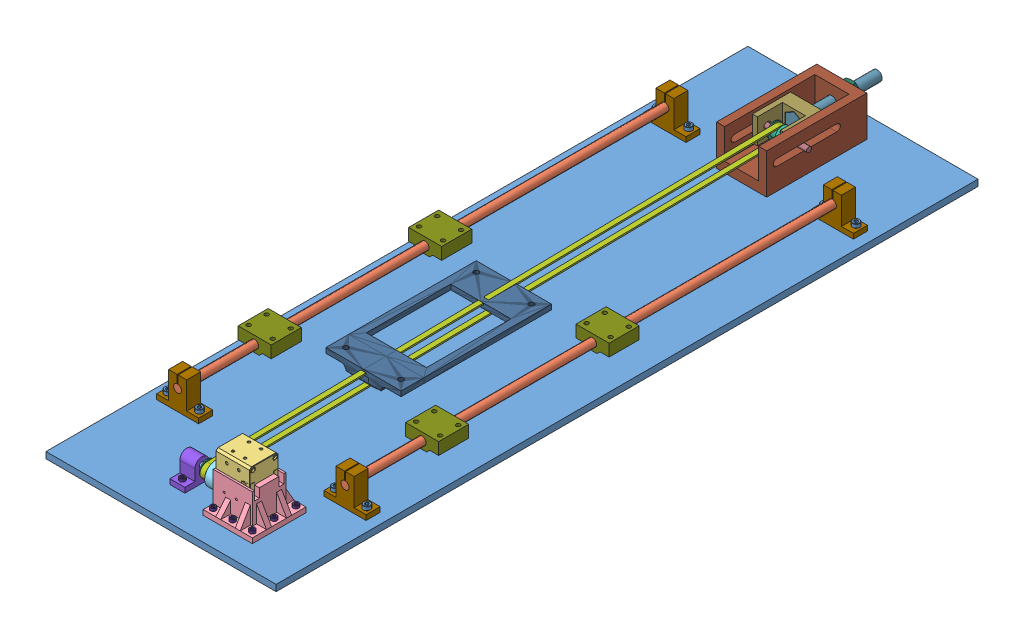
SolidWorks assembly linear_axis, configuration Défaut. Lengths in mm.
Overall size (229.5 66.71 714.21).
69 component instances, 25 part files, 88 mates.
Components (placement in the parent):
- plate-1: plate [Défaut] at origin size (229.5 6.35 700)
- rail-1: rail [Défaut] at (-83.5 26.35 250) x (-0.983228 -0.182381 0) z (0.182381 -0.983228 0) size (8 500 8)
- rail-2: rail [Défaut] at (83.5 26.35 250) x (0.983228 -0.182381 0) z (0.182381 0.983228 0) size (8 500 8)
- motor_case_pulley-1: motor_case_pulley [Défaut] at (16.75 22.6 300) x (0 0 1) z (-1 0 0) size (53.5 51.5 72)
  - XL430-W250-1: XL430-W250 [Défaut] at origin size (28.5 46.5 36.18)
  - motor_case-1: motor_case [Défaut] at (0 -16.25 -21.5) size (53.5 34.81 49)
  - coupler_pulley-2: coupler_pulley [Défaut] x (-1 0 0) z (0 1 0) size (22.5 12 20.75)
  - pulley-1: pulley [Défaut] at (0 0 21) x (1 0 0) z (0 1 0) size (15 16 15)
  - M2-4mm_TYPE 18-8 SS SOCKET HEAD CAP SCREW-1: M2-4mm_TYPE 18-8 SS SOCKET HEAD CAP SCREW [91292A832] at (-8 0 -2) x (-0.92231 0.38645 0) z (0 0 -1) size (3.8 3.8 6.09)
  - M2-4mm_TYPE 18-8 SS SOCKET HEAD CAP SCREW-2: M2-4mm_TYPE 18-8 SS SOCKET HEAD CAP SCREW [91292A832] at (0 8 -2) x (0.574993 -0.818158 0) z (0 0 -1) size (3.8 3.8 6.09)
  - M2-4mm_TYPE 18-8 SS SOCKET HEAD CAP SCREW-3: M2-4mm_TYPE 18-8 SS SOCKET HEAD CAP SCREW [91292A832] at (8 0 -2) x (-0.577346 0.816499 0) z (0 0 -1) size (3.8 3.8 6.09)
- pulley_axis_support-1: pulley_axis_support [Défaut] at (-9.25 22.6 300) x (0 0 1) z (0 -1 0) size (34 15 23)
- rail_support-5: rail_support [Défaut] at (-83.5 6.35 243) x (-1 0 0) z (0 0 -1) size (42 32 14)
- rail_support-6: rail_support [Défaut] at (83.5 6.35 243) x (-1 0 0) z (0 0 -1) size (42 32 14)
- rail_support-9: rail_support [Défaut] at (-83.5 6.35 -243) size (42 32 14)
- rail_support-10: rail_support [Défaut] at (83.5 6.35 -243) size (42 32 14)
- coupler_timing_belt_base-1: coupler_timing_belt_base [Défaut] at (37.5 33.85 148.1403) x (0 0 -1) z (-1 0 0) size (150 12 75)
- belt_tensioner-1: belt_tensioner [Défaut] at (70 26.35 -273.3415) x (0 0 1) z (-1 0 0) size (135.21 40 60)
  - tensioner_fixed_part-1: tensioner_fixed_part [Défaut] at (-5.6585 -20 70) size (100 40 50)
  - tensioner_moving_part-1: tensioner_moving_part [Défaut] at (17.1303 -7.5 53.5) size (38 25 33)
  - pulley-1: pulley [Défaut] at (7.1303 5 74.5) x (-0.489878 -0.871791 0) z (0.871791 -0.489878 0) size (15 16 15)
  - pulley_long_shaft-1: pulley_long_shaft [Défaut] at (7.1303 5 40) x (-0.998966 -0.045468 0) z (-0.045468 0.998966 0) size (5 60 5)
  - M10-75mm_TYPE 18-8 SS HEX HEAD CAP SCREW-1: M10-75mm_TYPE 18-8 SS HEX HEAD CAP SCREW [Défaut] at (-90.8697 5 70) x (0 -1 0) z (0 0 1) size (20 83 17.32)
  - M10-NUT_TYPE 18-8 SS THIN HEX NUT - DIN 439B (1)-1: M10-NUT_TYPE 18-8 SS THIN HEX NUT - DIN 439B (1) [Default] at (-55.6585 5 70) x (0 -0.532907 0.846174) z (0 -0.846174 -0.532907) size (17 10.59 19.63)
- linear_bearing-5: linear_bearing [Défaut] at (83.5 33.85 158.1403) x (-1 0 0) z (0 0 1) size (33 15 30)
- linear_bearing-6: linear_bearing [Défaut] at (83.5 33.85 -11.8597) x (-1 0 0) z (0 0 1) size (33 15 30)
- linear_bearing-7: linear_bearing [Défaut] at (-83.5 33.85 158.1403) x (1 0 0) z (0 0 -1) size (33 15 30)
- linear_bearing-8: linear_bearing [Défaut] at (-83.5 33.85 -11.8597) x (1 0 0) z (0 0 -1) size (33 15 30)
- M3-16mm_91292A115_TYPE 18-8 SS SOCKET HEAD CAP SCREW-1: M3-16mm_91292A115_TYPE 18-8 SS SOCKET HEAD CAP SCREW [91292A115] at (62.75 -4.65 321.75) x (0.995023 0 -0.099645) z (0 -1 0) size (5.5 5.5 19.25)
- M3-NUT_90710A030_TYPE 18-8 SS THIN HEX NUT - DIN 439B-1: M3-NUT_90710A030_TYPE 18-8 SS THIN HEX NUT - DIN 439B [90710A030] at (62.75 -0.9 321.75) x (0.992789 0 0.119878) z (-0.119878 0 0.992789) size (5.5 2.19 6.35)
- M3-NUT_90710A030_TYPE 18-8 SS THIN HEX NUT - DIN 439B-2: M3-NUT_90710A030_TYPE 18-8 SS THIN HEX NUT - DIN 439B [90710A030] at (43.25 -0.9 321.75) x (0.992789 0 0.119878) z (-0.119878 0 0.992789) size (5.5 2.19 6.35)
- M3-NUT_90710A030_TYPE 18-8 SS THIN HEX NUT - DIN 439B-3: M3-NUT_90710A030_TYPE 18-8 SS THIN HEX NUT - DIN 439B [90710A030] at (23.75 -0.9 321.75) x (0.992789 0 0.119878) z (-0.119878 0 0.992789) size (5.5 2.19 6.35)
- M3-16mm_91292A115_TYPE 18-8 SS SOCKET HEAD CAP SCREW-2: M3-16mm_91292A115_TYPE 18-8 SS SOCKET HEAD CAP SCREW [91292A115] at (43.25 -4.65 321.75) x (0.995023 0 -0.099645) z (0 -1 0) size (5.5 5.5 19.25)
- M3-16mm_91292A115_TYPE 18-8 SS SOCKET HEAD CAP SCREW-3: M3-16mm_91292A115_TYPE 18-8 SS SOCKET HEAD CAP SCREW [91292A115] at (23.75 -4.65 321.75) x (0.995023 0 -0.099645) z (0 -1 0) size (5.5 5.5 19.25)
- M3-NUT_90710A030_TYPE 18-8 SS THIN HEX NUT - DIN 439B-4: M3-NUT_90710A030_TYPE 18-8 SS THIN HEX NUT - DIN 439B [90710A030] at (62.75 -0.9 300) x (0.992789 0 0.119878) z (-0.119878 0 0.992789) size (5.5 2.19 6.35)
- M3-NUT_90710A030_TYPE 18-8 SS THIN HEX NUT - DIN 439B-5: M3-NUT_90710A030_TYPE 18-8 SS THIN HEX NUT - DIN 439B [90710A030] at (62.75 -0.9 278.25) x (0.992789 0 0.119878) z (-0.119878 0 0.992789) size (5.5 2.19 6.35)
- M3-16mm_91292A115_TYPE 18-8 SS SOCKET HEAD CAP SCREW-4: M3-16mm_91292A115_TYPE 18-8 SS SOCKET HEAD CAP SCREW [91292A115] at (62.75 -4.65 300) x (0.995023 0 -0.099645) z (0 -1 0) size (5.5 5.5 19.25)
- M3-16mm_91292A115_TYPE 18-8 SS SOCKET HEAD CAP SCREW-5: M3-16mm_91292A115_TYPE 18-8 SS SOCKET HEAD CAP SCREW [91292A115] at (62.75 -4.65 278.25) x (0.995023 0 -0.099645) z (0 -1 0) size (5.5 5.5 19.25)
- M3-NUT_90710A030_TYPE 18-8 SS THIN HEX NUT - DIN 439B-6: M3-NUT_90710A030_TYPE 18-8 SS THIN HEX NUT - DIN 439B [90710A030] at (43.25 -0.9 278.25) x (0.992789 0 0.119878) z (-0.119878 0 0.992789) size (5.5 2.19 6.35)
- M3-NUT_90710A030_TYPE 18-8 SS THIN HEX NUT - DIN 439B-7: M3-NUT_90710A030_TYPE 18-8 SS THIN HEX NUT - DIN 439B [90710A030] at (23.75 -0.9 278.25) x (0.992789 0 0.119878) z (-0.119878 0 0.992789) size (5.5 2.19 6.35)
- M3-16mm_91292A115_TYPE 18-8 SS SOCKET HEAD CAP SCREW-6: M3-16mm_91292A115_TYPE 18-8 SS SOCKET HEAD CAP SCREW [91292A115] at (43.25 -4.65 278.25) x (0.995023 0 -0.099645) z (0 -1 0) size (5.5 5.5 19.25)
- M3-16mm_91292A115_TYPE 18-8 SS SOCKET HEAD CAP SCREW-7: M3-16mm_91292A115_TYPE 18-8 SS SOCKET HEAD CAP SCREW [91292A115] at (23.75 -4.65 278.25) x (0.995023 0 -0.099645) z (0 -1 0) size (5.5 5.5 19.25)
- M3-16mm_91292A115_TYPE 18-8 SS SOCKET HEAD CAP SCREW-8: M3-16mm_91292A115_TYPE 18-8 SS SOCKET HEAD CAP SCREW [91292A115] at (-16.75 -4.4 312) x (0.715484 0 0.698629) z (0 -1 0) size (5.5 5.5 19.25)
- M3-NUT_90710A030_TYPE 18-8 SS THIN HEX NUT - DIN 439B-8: M3-NUT_90710A030_TYPE 18-8 SS THIN HEX NUT - DIN 439B [90710A030] at (-16.75 -0.9 312) size (5.5 2.19 6.35)
- M3-16mm_91292A115_TYPE 18-8 SS SOCKET HEAD CAP SCREW-9: M3-16mm_91292A115_TYPE 18-8 SS SOCKET HEAD CAP SCREW [91292A115] at (-16.75 -4.4 288) x (-0.715484 0 0.698629) z (0 -1 0) size (5.5 5.5 19.25)
- M3-NUT_90710A030_TYPE 18-8 SS THIN HEX NUT - DIN 439B-9: M3-NUT_90710A030_TYPE 18-8 SS THIN HEX NUT - DIN 439B [90710A030] at (-16.75 -0.9 288) size (5.5 2.19 6.35)
- M4-16mm_91292A118_TYPE 18-8 SS SOCKET HEAD CAP SCREW-1: M4-16mm_91292A118_TYPE 18-8 SS SOCKET HEAD CAP SCREW [91292A118] at (99.25 -4.65 244) x (0.684649 0 0.728873) z (0 -1 0) size (7 7 20.35)
- M4-16mm_91292A118_TYPE 18-8 SS SOCKET HEAD CAP SCREW-2: M4-16mm_91292A118_TYPE 18-8 SS SOCKET HEAD CAP SCREW [91292A118] at (67.75 -4.65 244) x (0.152759 0 0.988263) z (0 -1 0) size (7 7 20.35)
- M4-16mm_91292A118_TYPE 18-8 SS SOCKET HEAD CAP SCREW-3: M4-16mm_91292A118_TYPE 18-8 SS SOCKET HEAD CAP SCREW [91292A118] at (-99.25 -4.65 244) x (0.684649 0 -0.728873) z (0 -1 0) size (7 7 20.35)
- M4-16mm_91292A118_TYPE 18-8 SS SOCKET HEAD CAP SCREW-4: M4-16mm_91292A118_TYPE 18-8 SS SOCKET HEAD CAP SCREW [91292A118] at (-67.75 -4.65 244) x (0.152759 0 -0.988263) z (0 -1 0) size (7 7 20.35)
- M4-16mm_91292A118_TYPE 18-8 SS SOCKET HEAD CAP SCREW-5: M4-16mm_91292A118_TYPE 18-8 SS SOCKET HEAD CAP SCREW [91292A118] at (99.25 -4.65 -244) x (0.684649 0 -0.728873) z (0 -1 0) size (7 7 20.35)
- M4-16mm_91292A118_TYPE 18-8 SS SOCKET HEAD CAP SCREW-6: M4-16mm_91292A118_TYPE 18-8 SS SOCKET HEAD CAP SCREW [91292A118] at (67.75 -4.65 -244) x (-0.152759 0 0.988263) z (0 -1 0) size (7 7 20.35)
- M4-16mm_91292A118_TYPE 18-8 SS SOCKET HEAD CAP SCREW-7: M4-16mm_91292A118_TYPE 18-8 SS SOCKET HEAD CAP SCREW [91292A118] at (-99.25 -4.65 -244) x (-0.684649 0 -0.728873) z (0 -1 0) size (7 7 20.35)
- M4-16mm_91292A118_TYPE 18-8 SS SOCKET HEAD CAP SCREW-8: M4-16mm_91292A118_TYPE 18-8 SS SOCKET HEAD CAP SCREW [91292A118] at (-67.75 -4.65 -244) x (-0.152759 0 -0.988263) z (0 -1 0) size (7 7 20.35)
- M5-20mm_TYPE 18-8 SS SOCKET HEAD CAP SCREW-1: M5-20mm_TYPE 18-8 SS SOCKET HEAD CAP SCREW [91292A118] at (0 -8.65 -304) x (0.974897 0 -0.222657) z (0 -1 0) size (9 9 24.44)
- M5-20mm_TYPE 18-8 SS SOCKET HEAD CAP SCREW-2: M5-20mm_TYPE 18-8 SS SOCKET HEAD CAP SCREW [91292A118] at (0 -8.65 -279) x (0.302619 0 0.953112) z (0 -1 0) size (9 9 24.44)
- M4-NUT_90710A035_TYPE 18-8 SS THIN HEX NUT - DIN 439B-9: M4-NUT_90710A035_TYPE 18-8 SS THIN HEX NUT - DIN 439B [90710A035] at (99.25 -1.1 244) x (0.723417 0 0.690412) z (-0.690412 0 0.723417) size (7 2.75 8.08)
- M4-NUT_90710A035_TYPE 18-8 SS THIN HEX NUT - DIN 439B-10: M4-NUT_90710A035_TYPE 18-8 SS THIN HEX NUT - DIN 439B [90710A035] at (67.75 -1.1 244) x (0.272287 0 0.962216) z (-0.962216 0 0.272287) size (7 2.75 8.08)
- M4-NUT_90710A035_TYPE 18-8 SS THIN HEX NUT - DIN 439B-11: M4-NUT_90710A035_TYPE 18-8 SS THIN HEX NUT - DIN 439B [90710A035] at (-99.25 -1.1004 244) x (-0.723417 0 0.690412) z (0.690412 0 0.723417) size (7 2.75 8.08)
- M4-NUT_90710A035_TYPE 18-8 SS THIN HEX NUT - DIN 439B-12: M4-NUT_90710A035_TYPE 18-8 SS THIN HEX NUT - DIN 439B [90710A035] at (-67.75 -1.1004 244) x (-0.272287 0 0.962216) z (0.962216 0 0.272287) size (7 2.75 8.08)
- M4-NUT_90710A035_TYPE 18-8 SS THIN HEX NUT - DIN 439B-13: M4-NUT_90710A035_TYPE 18-8 SS THIN HEX NUT - DIN 439B [90710A035] at (99.25 -1.1004 -244) x (0.723417 0 -0.690412) z (-0.690412 0 -0.723417) size (7 2.75 8.08)
- M4-NUT_90710A035_TYPE 18-8 SS THIN HEX NUT - DIN 439B-14: M4-NUT_90710A035_TYPE 18-8 SS THIN HEX NUT - DIN 439B [90710A035] at (67.75 -1.1004 -244) x (0.272287 0 -0.962216) z (-0.962216 0 -0.272287) size (7 2.75 8.08)
- M4-NUT_90710A035_TYPE 18-8 SS THIN HEX NUT - DIN 439B-15: M4-NUT_90710A035_TYPE 18-8 SS THIN HEX NUT - DIN 439B [90710A035] at (-67.75 -1.1 -244) x (-0.272287 0 -0.962216) z (0.962216 0 -0.272287) size (7 2.75 8.08)
- M4-NUT_90710A035_TYPE 18-8 SS THIN HEX NUT - DIN 439B-16: M4-NUT_90710A035_TYPE 18-8 SS THIN HEX NUT - DIN 439B [90710A035] at (-99.25 -1.1 -244) x (-0.723417 0 -0.690412) z (0.690412 0 -0.723417) size (7 2.75 8.08)
- M5-NUT_TYPE 18-8 SS THIN HEX NUT - DIN 439B-9: M5-NUT_TYPE 18-8 SS THIN HEX NUT - DIN 439B [90710A035] at (0 -1.5 -304) x (0.987172 0 -0.159659) z (0.159659 0 0.987172) size (8 3.55 9.24)
- M5-NUT_TYPE 18-8 SS THIN HEX NUT - DIN 439B-10: M5-NUT_TYPE 18-8 SS THIN HEX NUT - DIN 439B [90710A035] at (0 -1.5 -279) size (8 3.55 9.24)
- pulley_shaft-1: pulley_shaft [Défaut] at (-23.4279 22.6 300) x (0 -0.50423 0.863569) z (0 0.863569 0.50423) size (5 40 5)
- M4-8mm_91292A108_TYPE 18-8 SS SOCKET HEAD CAP SCREW-1: M4-8mm_91292A108_TYPE 18-8 SS SOCKET HEAD CAP SCREW [91292A108] at (7.75 20.1 300) x (0.999637 0 -0.026942) z (0 1 0) size (7 7 12.31)
- timing_belt-1: timing_belt [Défaut] at (0 26.9744 17.7551) x (0 -0.015407 0.999881) z (1 0 0) size (582 14 5)
Mates (geometry in assembly coordinates):
- Parallèle2: parallel aligned: plane of plaque-1 through (114.75 6.35 -350) normal (1 0 0); plane of robot_base_plate-1 through (100 35.85 -91.2538) normal (1 0 0)
- Parallèle3: parallel anti-aligned: plane of plaque-1 through (0 6.35 0) normal (0 1 0); plane of robot_base_plate-1 through (0 33.85 8.7462) normal (0 -1 0)
- Largeur1: width anti-aligned: plane of robot_base_plate-1 through (100 35.85 -91.2538) normal (1 0 0); plane of plaque-1 through (-100 35.85 -91.2538) normal (-1 0 0); plane of robot_base_plate-1 through (-114.75 6.35 -350) normal (-1 0 0); plane of plaque-1 through (114.75 6.35 -350) normal (1 0 0)
- Coïncidente4: coincident anti-aligned: plane of robot_base_plate-1 through (0 33.85 8.7462) normal (0 -1 0); plane of linear_bearing-1 through (131.2296 66.0945 93.7462) normal (0 1 0)
- Coïncidente5: coincident: point of robot_base_plate-1; unknown of linear_bearing-1
- Coïncidente6: coincident aligned: plane of robot_base_plate-1 through (-100 35.85 108.7462) normal (0 0 1); plane of linear_bearing-1 through (114.7296 51.0945 108.7462) normal (0 0 1)
- Parallèle4: parallel aligned: plane of plaque-1 through (114.75 6.35 350) normal (0 0 1); plane of rail_cylindre-1 through (-83.5 26.35 250) normal (0 0 1)
- Coaxiale1: concentric aligned: circle of bearing_lineaire-2; circle of rail_cylindre-1
- Largeur2: width anti-aligned: plane of rail-1 through (-83.5 26.35 250) normal (0 0 1); plane of plaque-1 through (-83.5 26.35 -250) normal (0 0 -1); plane of rail-1 through (114.75 6.35 -350) normal (0 0 -1); plane of plaque-1 through (114.75 6.35 350) normal (0 0 1)
- Parallèle5: parallel: plane of plaque-1 through (-114.75 6.35 -350) normal (-1 0 0); line of moteuretsupport-1/support moteur-1 through (18.75 6.35 273.25) axis (0 0 1)
- Coïncidente15: coincident anti-aligned: plane of plaque-1 through (0 6.35 0) normal (0 1 0); plane of moteuretsupport-1/support moteur-1 through (38.25 6.35 300) normal (0 -1 0)
- Distance1: distance = 47 mm aligned: plane of plaque-1 through (114.75 6.35 -350) normal (1 0 0); plane of moteuretsupport-1/support moteur-1 through (67.75 11.35 273.25) normal (1 0 0)
- Distance2: distance = 50 mm: unknown of moteuretsupport-1/support moteur-1; line of plaque-1 through (-114.75 6.35 350) axis (1 0 0)
- Parallèle6: parallel anti-aligned: plane of plaque-1 through (0 6.35 0) normal (0 1 0); plane of support_axe_poulie-1 through (-24.25 6.6 283) normal (0 -1 0)
- Coaxiale2: concentric anti-aligned: circle of moteuretsupport-1/poulie-1; circle of support_axe_poulie-1
- Distance3: distance = 5 mm anti-aligned: plane of support_axe_poulie-1 through (-9.25 22.6 300) normal (1 0 0); plane of moteuretsupport-1/poulie-1 through (-4.25 22.6 300) normal (-1 0 0)
- Coïncidente19: coincident aligned: circle of rail_cylindre-1; circle of support_rail-5
- Coïncidente21: coincident anti-aligned: circle of plaque-1; circle of support_rail-5
- Coïncidente23: coincident aligned: circle of rail_cylindre-2; circle of support_rail-6
- Coïncidente24: coincident anti-aligned: circle of plaque-1; circle of support_rail-6
- Coïncidente25: coincident anti-aligned: circle of plaque-1; circle of support_rail-10
- Coïncidente26: coincident anti-aligned: circle of plaque-1; circle of support_rail-9
- Coïncidente28: coincident anti-aligned: circle of rail_cylindre-2; circle of support_rail-10
- Coïncidente30: coincident anti-aligned: circle of rail_cylindre-1; circle of support_rail-9
- Parallèle7: parallel anti-aligned: plane of robot_base_plate-1 through (-100 35.85 -91.2538) normal (0 0 -1); plane of coupler_timing_belt_base-1 through (37.5 33.85 148.1403) normal (0 0 1)
- Coïncidente32: coincident anti-aligned: plane of robot_base_plate-1 through (0 33.85 8.7462) normal (0 -1 0); plane of coupler_timing_belt_base-1 through (37.5 33.85 148.1403) normal (0 1 0)
- Largeur3: width anti-aligned: plane of coupler_timing_belt_base-1 through (37.5 33.85 -1.8597) normal (0 0 -1); plane of robot_base_plate-1 through (37.5 33.85 148.1403) normal (0 0 1); plane of coupler_timing_belt_base-1 through (-100 35.85 108.7462) normal (0 0 1); plane of robot_base_plate-1 through (-100 35.85 -91.2538) normal (0 0 -1)
- Largeur4: width anti-aligned: plane of coupler_timing_belt_base-1 through (37.5 33.85 148.1403) normal (1 0 0); plane of robot_base_plate-1 through (-37.5 33.85 148.1403) normal (-1 0 0); plane of coupler_timing_belt_base-1 through (-100 35.85 -91.2538) normal (-1 0 0); plane of robot_base_plate-1 through (100 35.85 -91.2538) normal (1 0 0)
- Parallèle9: parallel aligned: plane of plate-1 through (114.75 6.35 -350) normal (1 0 0); plane of belt_tensioner-1/tensioner_fixed_part-1 through (25 16.35 -329) normal (1 0 0)
- Coïncidente35: coincident anti-aligned: plane of plate-1 through (0 6.35 0) normal (0 1 0); plane of belt_tensioner-1/tensioner_fixed_part-1 through (0 6.35 -279) normal (0 -1 0)
- Coaxiale3: concentric aligned: cylinder of plate-1 through (0 0 -304) axis (0 1 0) radius 2.75; cylinder of belt_tensioner-1/tensioner_fixed_part-1 through (0 16.35 -304) axis (0 1 0) radius 2.75
- Coïncidente36: coincident anti-aligned: line of linear_bearing-1 through (147.7296 66.0945 78.7462) axis (0 0 1); line of Base_Robot-1 through (147.7296 66.0945 104.9261) axis (0 0 -1)
- Coaxiale4: concentric aligned: cylinder of rail-2 through (83.5 26.35 -250) axis (0 0 1) radius 4; circle of linear_bearing-5
- Parallèle10: parallel aligned: plane of plate-1 through (0 6.35 0) normal (0 1 0); plane of linear_bearing-5 through (83.5 33.85 158.1403) normal (0 1 0)
- Parallèle11: parallel aligned: plane of plate-1 through (0 6.35 0) normal (0 1 0); plane of linear_bearing-6 through (83.5 33.85 -11.8597) normal (0 1 0)
- Coaxiale5: concentric aligned: cylinder of rail-2 through (83.5 26.35 -250) axis (0 0 1) radius 4; cylinder of linear_bearing-6 through (83.5 26.35 -26.8597) axis (0 0 1) radius 4
- Coïncidente41: coincident anti-aligned: line of linear_bearing-5 through (100 33.85 143.1403) axis (0 0 1); line of robot_base_plate-2 through (100 33.85 70.7474) axis (0 0 -1)
- Coïncidente42: coincident anti-aligned: plane of linear_bearing-8 through (-83.5 33.85 -11.8597) normal (0 1 0); plane of robot_base_plate-2 through (0 33.85 -29.2526) normal (0 -1 0)
- Coïncidente43: coincident anti-aligned: line of linear_bearing-8 through (-100 33.85 -26.8597) axis (1 0 0); line of robot_base_plate-2 through (100 33.85 -129.2526) axis (-1 0 0)
- Coïncidente44: coincident anti-aligned: line of linear_bearing-7 through (-67 33.85 173.1403) axis (-1 0 0); line of robot_base_plate-2 through (-100 33.85 70.7474) axis (1 0 0)
- Coïncidente45: coincident anti-aligned: plane of coupler_timing_belt_base-1 through (37.5 33.85 148.1403) normal (0 1 0); plane of Base_Robot-2 through (0 33.85 -29.2526) normal (0 -1 0)
- Largeur5: width anti-aligned: plane of coupler_timing_belt_base-1 through (-37.5 33.85 148.1403) normal (-1 0 0); plane of coupler_timing_belt_base-1 through (37.5 33.85 148.1403) normal (1 0 0); plane of Base_Robot-2 through (100 35.85 70.7474) normal (1 0 0); plane of Base_Robot-2 through (-100 35.85 70.7474) normal (-1 0 0)
- Largeur6: width anti-aligned: plane of coupler_timing_belt_base-1 through (37.5 33.85 -1.8597) normal (0 0 -1); plane of coupler_timing_belt_base-1 through (37.5 33.85 148.1403) normal (0 0 1); plane of Base_Robot-2 through (100 35.85 70.7474) normal (0 0 1); plane of Base_Robot-2 through (100 35.85 -129.2526) normal (0 0 -1)
- Coïncidente47: coincident aligned: plane of coupler_timing_belt_base-1 through (37.5 33.85 148.1403) normal (0 1 0); plane of linear_bearing-7 through (-83.5 33.85 158.1403) normal (0 1 0)
- Largeur7: width anti-aligned: plane of coupler_timing_belt_base-1 through (37.5 33.85 148.1403) normal (1 0 0); plane of plate-1 through (-37.5 33.85 148.1403) normal (-1 0 0); plane of coupler_timing_belt_base-1 through (-114.75 6.35 -350) normal (-1 0 0); plane of plate-1 through (114.75 6.35 -350) normal (1 0 0)
- Distance4: distance = 200 mm: line of linear_bearing-7 through (-67 33.85 173.1403) axis (-1 0 0); line of linear_bearing-8 through (-100 33.85 -26.8597) axis (1 0 0)
- Largeur8: width anti-aligned: plane of coupler_timing_belt_base-1 through (37.5 33.85 148.1403) normal (0 0 1); plane of linear_bearing-6 through (37.5 33.85 -1.8597) normal (0 0 -1); plane of coupler_timing_belt_base-1 through (67 18.85 -26.8597) normal (0 0 -1); plane of linear_bearing-5 through (67 18.85 173.1403) normal (0 0 1)
- Coaxiale6: concentric anti-aligned: cylinder of motor_case_pulley-1/motor_case-1 through (62.75 6.35 321.75) axis (0 1 0) radius 2; cylinder of M3-12mm_91292A114_TYPE 18-8 SS SOCKET HEAD CAP SCREW-1 through (62.75 19.8774 321.75) axis (0 -1 0) radius 2.75
- Coaxiale7: concentric anti-aligned: cylinder of motor_case_pulley-1/motor_case-1 through (62.75 6.35 321.75) axis (0 1 0) radius 2; cylinder of M3-16mm_91292A115_TYPE 18-8 SS SOCKET HEAD CAP SCREW-1 through (62.75 14.35 321.75) axis (0 -1 0) radius 2.75
- Coïncidente50: coincident anti-aligned: plane of motor_case_pulley-1/motor_case-1 through (38.25 11.35 300) normal (0 1 0); plane of M3-16mm_91292A115_TYPE 18-8 SS SOCKET HEAD CAP SCREW-1 through (62.75 11.35 321.75) normal (0 -1 0)
- Coaxiale8: concentric anti-aligned: circle of plate-1; circle of M3-NUT_90710A030_TYPE 18-8 SS THIN HEX NUT - DIN 439B-1
- Coïncidente51: coincident anti-aligned: plane of plate-1 through (0 0 0) normal (0 -1 0); plane of M3-NUT_90710A030_TYPE 18-8 SS THIN HEX NUT - DIN 439B-1 through (60.2102 0 319.8441) normal (0 1 0)
- Coaxiale9: concentric anti-aligned: cylinder of pulley_axis_support-1 through (-16.75 -3.4 312) axis (0 1 0) radius 2; cylinder of M3-16mm_91292A115_TYPE 18-8 SS SOCKET HEAD CAP SCREW-8 through (-16.75 14.6 312) axis (0 -1 0) radius 2.75
- Coïncidente52: coincident anti-aligned: plane of pulley_axis_support-1 through (-24.25 11.6 307) normal (0 1 0); plane of M3-16mm_91292A115_TYPE 18-8 SS SOCKET HEAD CAP SCREW-8 through (-16.75 11.6 312) normal (0 -1 0)
- Coïncidente53: coincident anti-aligned: cylinder of M3-16mm_91292A115_TYPE 18-8 SS SOCKET HEAD CAP SCREW-8 through (-16.75 14.6 312) axis (0 -1 0) radius 2.75; circle of M3-NUT_90710A030_TYPE 18-8 SS THIN HEX NUT - DIN 439B-8
- Coïncidente54: coincident anti-aligned: plane of plate-1 through (0 0 0) normal (0 -1 0); plane of M3-NUT_90710A030_TYPE 18-8 SS THIN HEX NUT - DIN 439B-8 through (-19.5 0 310.4123) normal (0 1 0)
- Coaxiale10: concentric anti-aligned: cylinder of rail_support-6 through (99.25 6.35 244) axis (0 1 0) radius 2.5; cylinder of M4-16mm_91292A118_TYPE 18-8 SS SOCKET HEAD CAP SCREW-1 through (99.25 15.35 244) axis (0 -1 0) radius 3.5
- Coïncidente55: coincident anti-aligned: plane of rail_support-6 through (104.5 11.35 250) normal (0 1 0); plane of M4-16mm_91292A118_TYPE 18-8 SS SOCKET HEAD CAP SCREW-1 through (99.25 11.35 244) normal (0 -1 0)
- Coaxiale11: concentric anti-aligned: cylinder of rail_support-6 through (67.75 6.35 244) axis (0 1 0) radius 2.5; cylinder of M4-16mm_91292A118_TYPE 18-8 SS SOCKET HEAD CAP SCREW-2 through (67.75 15.35 244) axis (0 -1 0) radius 3.5
- Coïncidente56: coincident anti-aligned: plane of rail_support-6 through (62.5 11.35 250) normal (0 1 0); plane of M4-16mm_91292A118_TYPE 18-8 SS SOCKET HEAD CAP SCREW-2 through (67.75 11.35 244) normal (0 -1 0)
- Coaxiale12: concentric anti-aligned: cylinder of M4-16mm_91292A118_TYPE 18-8 SS SOCKET HEAD CAP SCREW-1 through (99.25 15.35 244) axis (0 -1 0) radius 3.5; circle of M4-NUT_90710A035_TYPE 18-8 SS THIN HEX NUT - DIN 439B-2
- Coïncidente58: coincident: cylinder of M4-16mm_91292A118_TYPE 18-8 SS SOCKET HEAD CAP SCREW-2 through (67.75 15.35 244) axis (0 -1 0) radius 3.5; circle of M4-NUT_90710A035_TYPE 18-8 SS THIN HEX NUT - DIN 439B-1
- Coïncidente59: coincident anti-aligned: plane of plate-1 through (0 0 0) normal (0 -1 0); plane of M5-NUT_TYPE 18-8 SS THIN HEX NUT - DIN 439B-2 through (95.9545 0 240.7638) normal (0 1 0)
- Coïncidente60: coincident: plane of plate-1 through (0 0 0) normal (0 -1 0); plane of M4-NUT_90710A035_TYPE 18-8 SS THIN HEX NUT - DIN 439B-1 through (63.75 0.4 241.6905) normal (0 1 0)
- Coaxiale14: concentric anti-aligned: cylinder of belt_tensioner-1/tensioner_fixed_part-1 through (0 16.35 -304) axis (0 1 0) radius 5; cylinder of M5-20mm_TYPE 18-8 SS SOCKET HEAD CAP SCREW-1 through (0 15.35 -304) axis (0 -1 0) radius 4.5
- Coïncidente62: coincident anti-aligned: plane of belt_tensioner-1/tensioner_fixed_part-1 through (0 11.35 -301.25) normal (0 1 0); plane of M5-20mm_TYPE 18-8 SS SOCKET HEAD CAP SCREW-1 through (0 11.35 -304) normal (0 -1 0)
- Coaxiale15: concentric anti-aligned: cylinder of belt_tensioner-1/tensioner_fixed_part-1 through (0 16.35 -279) axis (0 1 0) radius 5; cylinder of M5-20mm_TYPE 18-8 SS SOCKET HEAD CAP SCREW-2 through (0 15.35 -279) axis (0 -1 0) radius 4.5
- Coïncidente63: coincident anti-aligned: plane of belt_tensioner-1/tensioner_fixed_part-1 through (0 11.35 -276.25) normal (0 1 0); plane of M5-20mm_TYPE 18-8 SS SOCKET HEAD CAP SCREW-2 through (0 11.35 -279) normal (0 -1 0)
- Coïncidente64: coincident anti-aligned: cylinder of M4-16mm_91292A118_TYPE 18-8 SS SOCKET HEAD CAP SCREW-1 through (99.25 15.35 244) axis (0 -1 0) radius 3.5; circle of M4-NUT_90710A035_TYPE 18-8 SS THIN HEX NUT - DIN 439B-9
- Coïncidente65: coincident anti-aligned: plane of plate-1 through (0 0 0) normal (0 -1 0); plane of M4-NUT_90710A035_TYPE 18-8 SS THIN HEX NUT - DIN 439B-9 through (98.1132 0 240.1217) normal (0 1 0)
- Coïncidente66: coincident anti-aligned: cylinder of M4-16mm_91292A118_TYPE 18-8 SS SOCKET HEAD CAP SCREW-2 through (67.75 15.35 244) axis (0 -1 0) radius 3.5; circle of M4-NUT_90710A035_TYPE 18-8 SS THIN HEX NUT - DIN 439B-10
- Coïncidente67: coincident anti-aligned: plane of plate-1 through (0 0 0) normal (0 -1 0); plane of M4-NUT_90710A035_TYPE 18-8 SS THIN HEX NUT - DIN 439B-10 through (68.7414 0 240.082) normal (0 1 0)
- Coaxiale16: concentric aligned: circle of plate-1; circle of M5-NUT_TYPE 18-8 SS THIN HEX NUT - DIN 439B-9
- Coïncidente68: coincident anti-aligned: plane of plate-1 through (0 0 0) normal (0 -1 0); plane of M5-NUT_TYPE 18-8 SS THIN HEX NUT - DIN 439B-9 through (-4.3174 0 -305.6411) normal (0 1 0)
- Coïncidente69: coincident anti-aligned: plane of plate-1 through (0 0 0) normal (0 -1 0); plane of M5-NUT_TYPE 18-8 SS THIN HEX NUT - DIN 439B-10 through (-4 0 -281.3094) normal (0 1 0)
- Coaxiale17: concentric anti-aligned: circle of plate-1; circle of M5-NUT_TYPE 18-8 SS THIN HEX NUT - DIN 439B-10
- Coaxiale18: concentric anti-aligned: cylinder of pulley_axis_support-1 through (-24.25 22.6 300) axis (1 0 0) radius 2.5; cylinder of pulley_shaft-1 through (16.5721 22.6 300) axis (-1 0 0) radius 2.5
- Coïncidente70: coincident anti-aligned: plane of motor_case_pulley-1/XL430-W250-1 through (16.5721 27.1585 295) normal (-1 0 0); plane of pulley_shaft-1 through (16.5721 22.6 300) normal (1 0 0)
- Coaxiale19: concentric anti-aligned: cylinder of motor_case_pulley-1/coupler_pulley-2 through (7.75 23.1 300) axis (0 -1 0) radius 2; cylinder of M4-8mm_91292A108_TYPE 18-8 SS SOCKET HEAD CAP SCREW-1 through (7.75 8.1 300) axis (0 1 0) radius 3.5
- Tangent1: tangent anti-aligned: cylinder of pulley_shaft-1 through (16.5721 22.6 300) axis (-1 0 0) radius 2.5; plane of M4-8mm_91292A108_TYPE 18-8 SS SOCKET HEAD CAP SCREW-1 through (7.75 20.1 300) normal (0 1 0)
- Coaxiale20: concentric aligned: cylinder of belt_tensioner-1/tensioner_fixed_part-1 through (0 31.35 -229) axis (0 0 -1) radius 5.25; cylinder of M10-75mm_TYPE 18-8 SS HEX HEAD CAP SCREW-1 through (0 31.35 -290.6137) axis (0 0 -1) radius 5
- Coïncidente72: coincident anti-aligned: plane of belt_tensioner-1/tensioner_moving_part-1 through (16.5 18.85 -289.2112) normal (0 0 1); plane of M10-75mm_TYPE 18-8 SS HEX HEAD CAP SCREW-1 through (0 31.35 -290.6137) normal (0 0 -1)
- Parallèle12: parallel anti-aligned: plane of belt_tensioner-1/tensioner_moving_part-1 through (9.0933 36.6 -289.2112) normal (-0.5 -0.866025 0); plane of M10-75mm_TYPE 18-8 SS HEX HEAD CAP SCREW-1 through (0 41.35 -282.6137) normal (0.5 0.866025 0)
- Coaxiale21: concentric: cylinder of M10-75mm_TYPE 18-8 SS HEX HEAD CAP SCREW-1 through (0 31.35 -290.6137) axis (0 0 -1) radius 5; circle of M10-NUT_TYPE 18-8 SS THIN HEX NUT - DIN 439B (1)-1
- Coïncidente74: coincident anti-aligned: plane of belt_tensioner-1/tensioner_fixed_part-1 through (-25 16.35 -329) normal (0 0 -1); plane of M10-NUT_TYPE 18-8 SS THIN HEX NUT - DIN 439B (1)-1 through (0 31.35 -329) normal (0 0 1)
- Coaxiale22: concentric anti-aligned: cylinder of belt_tensioner-1/pulley-1 through (-4.5 31.35 -266.2112) axis (-1 0 0) radius 5.5; cylinder of timing_belt-1 through (-2.5 31.35 -266.2112) axis (1 0 0) radius 5.5
- Largeur9: width aligned: plane of timing_belt-1 through (2.5 22.5988 301.7214) normal (1 0 0); plane of timing_belt-1 through (-2.5 22.5988 301.7214) normal (-1 0 0); plane of belt_tensioner-1/pulley-1 through (-3.5 27.6759 -259.6727) normal (1 0 0); plane of belt_tensioner-1/pulley-1 through (3.5 27.6759 -259.6727) normal (-1 0 0)
- Distance5: distance = 9.2497 mm: line of timing_belt-1 through (-2.5 15.5997 301.6136) axis (1 0 0); plane of plate-1 through (0 6.35 0) normal (0 1 0)
